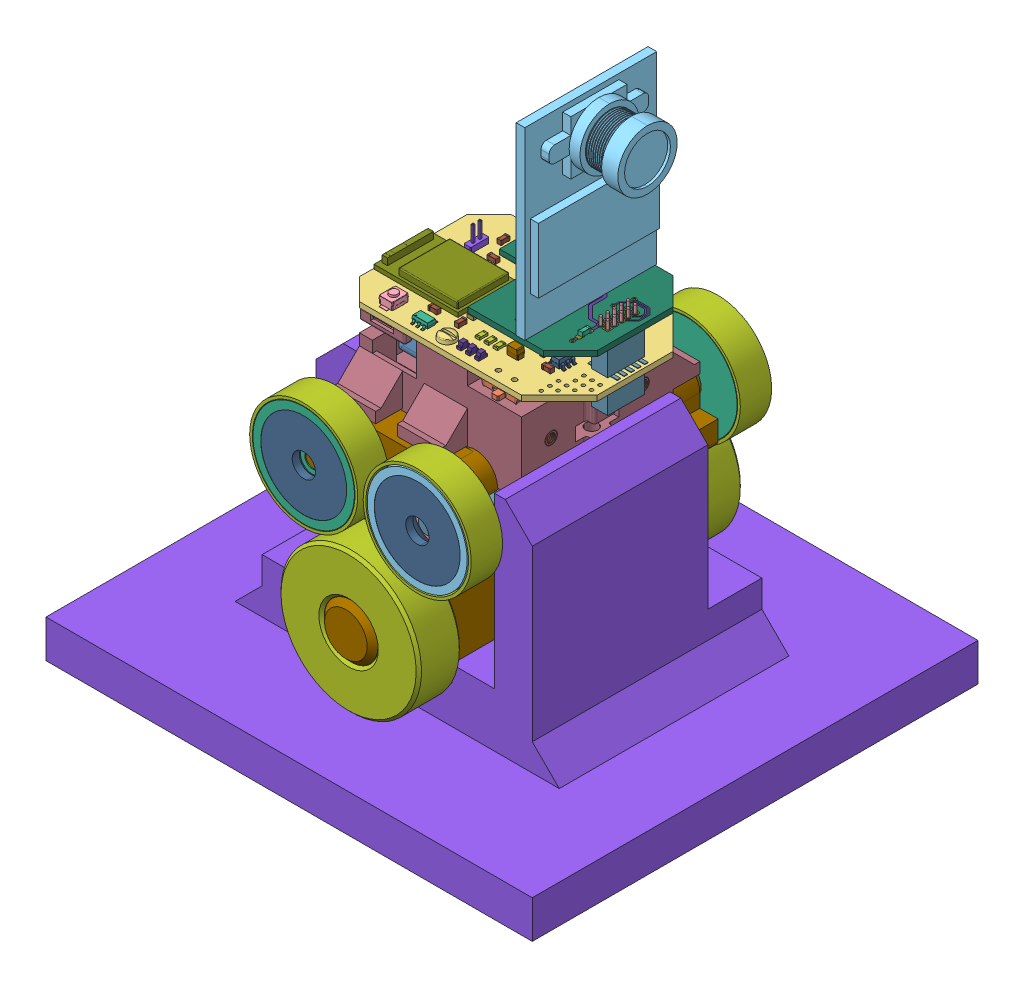
SolidWorks assembly life_time_test, configuration Default. Lengths in mm.
Overall size (90 100.86 82.5).
164 component instances, 45 part files, 11 mates.
Components (placement in the parent):
- AstroAnt_small_magnet-1: AstroAnt_small_magnet [Default] at (33.8115 12.6549 0.8712) size (45.75 69.7 55.6)
  - LiPo_360mAh-1: LiPo_360mAh [Default] at (6.8166 4.9998 44.2756) size (25 7 18)
  - 92120A150_Brass Heat-Set Inserts for Plastic-1: 92120A150_Brass Heat-Set Inserts for Plastic [92120A150] at (19.9543 12.4998 45.7029) size (2.56 3.33 2.56)
  - 92120A150_Brass Heat-Set Inserts for Plastic-2: 92120A150_Brass Heat-Set Inserts for Plastic [92120A150] at (4.9543 12.4998 33.9529) size (2.56 3.33 2.56)
  - 92120A150_Brass Heat-Set Inserts for Plastic-3: 92120A150_Brass Heat-Set Inserts for Plastic [92120A150] at (4.9543 12.4998 57.4529) size (2.56 3.33 2.56)
  - 91460A005_METRIC CHEESE HEAD SLOTTED MACHINE SCREW-8: 91460A005_METRIC CHEESE HEAD SLOTTED MACHINE SCREW [91460A005] at (4.9543 14.9998 57.4529) x (1 0 0) z (0 1 0) size (3 3 7.1)
  - 91460A005_METRIC CHEESE HEAD SLOTTED MACHINE SCREW-9: 91460A005_METRIC CHEESE HEAD SLOTTED MACHINE SCREW [91460A005] at (4.9543 14.9998 33.9529) x (1 0 0) z (0 1 0) size (3 3 7.1)
  - 91460A005_METRIC CHEESE HEAD SLOTTED MACHINE SCREW-10: 91460A005_METRIC CHEESE HEAD SLOTTED MACHINE SCREW [91460A005] at (19.9543 14.9998 45.7029) x (1 0 0) z (0 1 0) size (3 3 7.1)
  - 92120A150_Brass Heat-Set Inserts for Plastic-4: 92120A150_Brass Heat-Set Inserts for Plastic [92120A150] at (4.9543 -0.6002 57.4529) x (-0.616962 0 -0.786993) z (0.786993 0 -0.616962) size (2.56 3.33 2.56)
  - 92120A150_Brass Heat-Set Inserts for Plastic-5: 92120A150_Brass Heat-Set Inserts for Plastic [92120A150] at (4.9543 -0.6002 33.9529) x (-0.616962 0 -0.786993) z (0.786993 0 -0.616962) size (2.56 3.33 2.56)
  - mainboard_v1.step-1: mainboard_v1.step [Default] at (-103.0457 13.9998 235.7029) x (0 0 -1) z (0 1 0) size (29.41 41 10.8)
    - B3U-1000P.step-1: B3U-1000P.step [Default] at (178.95 -97.38 1.05) x (1 0 0) z (0 -1 0) size (4 1.75 2.5)
      - COMPOUND.step-1: COMPOUND.step [Default] at origin size (4 1.75 2.5)
    - 20021321-00014C1LF.step-1: 20021321-00014C1LF.step [Default] at (190 -115.5 1.05) size (9.35 5.45 4.85)
      - COMPOUND-0.step-1: COMPOUND-0.step [Default] at origin size (9.35 5.45 4.85)
    - MP6513GJ-Z.step-1: MP6513GJ-Z.step [Default] at (201.21 -120 1.05) x (-1 0 0) z (0 0 1) size (2.8 2.9 1)
      - COMPOUND-1.step-1: COMPOUND-1.step [Default] at origin size (2.8 2.9 1)
    - MP6513GJ-Z.step-2: MP6513GJ-Z.step [Default] at (178.51 -103.46 1.05) size (2.8 2.9 1)
      - COMPOUND-1.step-1: COMPOUND-1.step [Default] at origin size (2.8 2.9 1)
    - R_0603_1608Metric.step-1: R_0603_1608Metric.step [Default] at (195.55 -104.38 -0.05) x (1 0 0) z (0 0 -1) size (1.6 0.8 0.45)
      - SOLID.step-1: SOLID.step [Default] at origin size (1.6 0.8 0.45)
    - R_0603_1608Metric.step-2: R_0603_1608Metric.step [Default] at (192.6 -99.86 -0.05) x (0 1 0) z (0 0 -1) size (1.6 0.8 0.45)
      - SOLID.step-1: SOLID.step [Default] at origin size (1.6 0.8 0.45)
    - PinHeader_2x01_P1.27mm_Vertical.step-1: PinHeader_2x01_P1.27mm_Vertical.step [Default] at (194.96 -96.07 1.05) size (3.4 1.27 6.3)
      - SOLID-2.step-1: SOLID-2.step [Default] at origin size (3.4 1.27 6.3)
    - TAJP106K010RNJ.step-1: TAJP106K010RNJ.step [Default] at (196.22 -98.14 -0.05) x (-1 0 0) z (0 0 -1) size (2.05 1.4 1.7)
      - COMPOUND-3.step-1: COMPOUND-3.step [Default] at origin size (2.05 1.4 1.7)
    - TAJP106K010RNJ.step-2: TAJP106K010RNJ.step [Default] at (181.68 -117.23 1.05) x (0 1 0) z (0 0 1) size (2.05 1.4 1.7)
      - COMPOUND-3.step-1: COMPOUND-3.step [Default] at origin size (2.05 1.4 1.7)
    - SOT-23-5.step-1: SOT-23-5.step [Default] at (195.38 -122.78 1.05) x (0 1 0) z (0 0 1) size (2.8 2.9 1.55)
      - SOLID-4.step-1: SOLID-4.step [Default] at origin size (2.8 2.9 1.55)
    - C_0603_1608Metric.step-1: C_0603_1608Metric.step [Default] at (192.91 -122.55 1.05) x (0 -1 0) z (0 0 1) size (1.6 0.8 0.8)
      - SOLID-5.step-1: SOLID-5.step [Default] at origin size (1.6 0.8 0.8)
    - C_0603_1608Metric.step-2: C_0603_1608Metric.step [Default] at (193.57 -119.76 1.05) size (1.6 0.8 0.8)
      - SOLID-5.step-1: SOLID-5.step [Default] at origin size (1.6 0.8 0.8)
    - ECS-.327-12.5-12-TR.step-1: ECS-.327-12.5-12-TR.step [Default] at (184.31 -107.18 1.05) size (2 1.2 0.7)
      - COMPOUND-6.step-1: COMPOUND-6.step [Default] at origin size (2 1.2 0.7)
    - C_0603_1608Metric.step-3: C_0603_1608Metric.step [Default] at (197.67 -113.69 1.05) size (1.6 0.8 0.8)
      - SOLID-5.step-1: SOLID-5.step [Default] at origin size (1.6 0.8 0.8)
    - C_0603_1608Metric.step-4: C_0603_1608Metric.step [Default] at (197.64 -107.18 1.05) size (1.6 0.8 0.8)
      - SOLID-5.step-1: SOLID-5.step [Default] at origin size (1.6 0.8 0.8)
    - C_0603_1608Metric.step-5: C_0603_1608Metric.step [Default] at (190.96 -108.09 1.05) x (0 1 0) z (0 0 1) size (1.6 0.8 0.8)
      - SOLID-5.step-1: SOLID-5.step [Default] at origin size (1.6 0.8 0.8)
    - 1734592-6.step-1: 1734592-6.step [Default] at (203.79 -118 -1.05) x (0 -1 0) z (1 0 0) size (8.43 2.05 5.11)
      - SOLID-7.step-1: SOLID-7.step [Default] at origin size (8.43 2.05 5.11)
    - 1734592-6.step-2: 1734592-6.step [Default] at (176.19 -98 -1.05) x (0 1 0) z (-1 0 0) size (8.43 2.05 5.11)
      - SOLID-7.step-1: SOLID-7.step [Default] at origin size (8.43 2.05 5.11)
    - 20021321-00010C4LF.step-1: 20021321-00010C4LF.step [Default] at (190 -127.85 -0.05) x (1 0 0) z (0 0 -1) size (6.81 5.45 4.85)
      - COMPOUND-8.step-1: COMPOUND-8.step [Default] at origin size (6.81 5.45 4.85)
    - 20021321-00010C4LF.step-2: 20021321-00010C4LF.step [Default] at (190 -127.85 1.05) size (6.81 5.45 4.85)
      - COMPOUND-8.step-1: COMPOUND-8.step [Default] at origin size (6.81 5.45 4.85)
    - C_0603_1608Metric.step-6: C_0603_1608Metric.step [Default] at (181.31 -102.6 1.05) x (0 -1 0) z (0 0 1) size (1.6 0.8 0.8)
      - SOLID-5.step-1: SOLID-5.step [Default] at origin size (1.6 0.8 0.8)
    - C_0603_1608Metric.step-7: C_0603_1608Metric.step [Default] at (198.25 -119.14 1.05) x (0 -1 0) z (0 0 1) size (1.6 0.8 0.8)
      - SOLID-5.step-1: SOLID-5.step [Default] at origin size (1.6 0.8 0.8)
    - MPU6050.step-1: MPU6050.step [Default] at (198.43 -101.5 1.05) x (0 1 0) z (1 0 0) size (4 0.95 4)
      - COMPOUND-9.step-1: COMPOUND-9.step [Default] at origin size (4 0.95 4)
    - C_0603_1608Metric.step-8: C_0603_1608Metric.step [Default] at (194.9 -99.89 1.05) x (0 -1 0) z (0 0 1) size (1.6 0.8 0.8)
      - SOLID-5.step-1: SOLID-5.step [Default] at origin size (1.6 0.8 0.8)
    - C_0603_1608Metric.step-9: C_0603_1608Metric.step [Default] at (201.98 -100.38 1.05) x (0 -1 0) z (0 0 1) size (1.6 0.8 0.8)
      - SOLID-5.step-1: SOLID-5.step [Default] at origin size (1.6 0.8 0.8)
    - C_0603_1608Metric.step-10: C_0603_1608Metric.step [Default] at (201.98 -103.78 1.05) x (0 1 0) z (0 0 1) size (1.6 0.8 0.8)
      - SOLID-5.step-1: SOLID-5.step [Default] at origin size (1.6 0.8 0.8)
    - C_0603_1608Metric.step-11: C_0603_1608Metric.step [Default] at (198.81 -97.82 1.05) size (1.6 0.8 0.8)
      - SOLID-5.step-1: SOLID-5.step [Default] at origin size (1.6 0.8 0.8)
    - SOT-23-5.step-2: SOT-23-5.step [Default] at (184.86 -122.77 1.05) x (0 1 0) z (0 0 1) size (2.8 2.9 1.55)
      - SOLID-4.step-1: SOLID-4.step [Default] at origin size (2.8 2.9 1.55)
    - SOT-23-5.step-3: SOT-23-5.step [Default] at (197.58 -110.46 1.05) x (0 1 0) z (0 0 1) size (2.8 2.9 1.55)
      - SOLID-4.step-1: SOLID-4.step [Default] at origin size (2.8 2.9 1.55)
    - MDBT50Q-1MV2.step-1: MDBT50Q-1MV2.step [Default] at (187.3136 -98.605 1.0754) x (-1 0 0) z (0 1 0) size (10.5 2.06 15.5)
      - SOLID-10.step-1: SOLID-10.step [Default] at origin size (10.5 2.06 15.5)
    - C_0603_1608Metric.step-12: C_0603_1608Metric.step [Default] at (189.44 -108.09 1.05) x (0 1 0) z (0 0 1) size (1.6 0.8 0.8)
      - SOLID-5.step-1: SOLID-5.step [Default] at origin size (1.6 0.8 0.8)
    - C_0603_1608Metric.step-13: C_0603_1608Metric.step [Default] at (181.57 -107.18 1.05) x (-1 0 0) z (0 0 1) size (1.6 0.8 0.8)
      - SOLID-5.step-1: SOLID-5.step [Default] at origin size (1.6 0.8 0.8)
    - C_0603_1608Metric.step-14: C_0603_1608Metric.step [Default] at (186.97 -107.18 1.05) size (1.6 0.8 0.8)
      - SOLID-5.step-1: SOLID-5.step [Default] at origin size (1.6 0.8 0.8)
    - C_0603_1608Metric.step-15: C_0603_1608Metric.step [Default] at (184.77 -119.75 1.05) x (-1 0 0) z (0 0 1) size (1.6 0.8 0.8)
      - SOLID-5.step-1: SOLID-5.step [Default] at origin size (1.6 0.8 0.8)
    - C_0603_1608Metric.step-16: C_0603_1608Metric.step [Default] at (182.37 -122.54 1.05) x (0 -1 0) z (0 0 1) size (1.6 0.8 0.8)
      - SOLID-5.step-1: SOLID-5.step [Default] at origin size (1.6 0.8 0.8)
    - LED_0603_1608Metric.step-1: LED_0603_1608Metric.step [Default] at (178.19 -111.01 1.05) size (1.6 0.8 1.1)
      - SOLID-11.step-1: SOLID-11.step [Default] at origin size (1.6 0.8 1.1)
    - LED_0603_1608Metric.step-2: LED_0603_1608Metric.step [Default] at (178.19 -112.66 1.05) size (1.6 0.8 1.1)
      - SOLID-11.step-1: SOLID-11.step [Default] at origin size (1.6 0.8 1.1)
    - LED_0603_1608Metric.step-3: LED_0603_1608Metric.step [Default] at (178.19 -114.31 1.05) size (1.6 0.8 1.1)
      - SOLID-11.step-1: SOLID-11.step [Default] at origin size (1.6 0.8 1.1)
    - LED_0603_1608Metric.step-4: LED_0603_1608Metric.step [Default] at (202.34 -112.21 1.05) x (0 1 0) z (0 0 1) size (1.6 0.8 1.1)
      - SOLID-11.step-1: SOLID-11.step [Default] at origin size (1.6 0.8 1.1)
    - 473460001.step-1: 473460001.step [Default] at (201.68 -99.72 -1.25) x (0 -1 0) z (1 0 0) size (7.98 2.94 5.43)
      - COMPOUND-12.step-1: COMPOUND-12.step [Default] at origin size (7.98 2.94 5.43)
    - L_0603_1608Metric.step-1: L_0603_1608Metric.step [Default] at (192.48 -108.09 1.05) x (0 1 0) z (0 0 1) size (1.6 0.8 0.8)
      - SOLID-13.step-1: SOLID-13.step [Default] at origin size (1.6 0.8 0.8)
    - R_0603_1608Metric.step-3: R_0603_1608Metric.step [Default] at (185.18 -111.31 1.05) x (-1 0 0) z (0 0 1) size (1.6 0.8 0.45)
      - SOLID.step-1: SOLID.step [Default] at origin size (1.6 0.8 0.45)
    - R_0603_1608Metric.step-4: R_0603_1608Metric.step [Default] at (185.18 -109.77 1.05) size (1.6 0.8 0.45)
      - SOLID.step-1: SOLID.step [Default] at origin size (1.6 0.8 0.45)
    - R_0603_1608Metric.step-5: R_0603_1608Metric.step [Default] at (181.62 -111.01 1.05) size (1.6 0.8 0.45)
      - SOLID.step-1: SOLID.step [Default] at origin size (1.6 0.8 0.45)
    - R_0603_1608Metric.step-6: R_0603_1608Metric.step [Default] at (181.62 -112.66 1.05) size (1.6 0.8 0.45)
      - SOLID.step-1: SOLID.step [Default] at origin size (1.6 0.8 0.45)
    - R_0603_1608Metric.step-7: R_0603_1608Metric.step [Default] at (181.62 -114.31 1.05) x (-1 0 0) z (0 0 1) size (1.6 0.8 0.45)
      - SOLID.step-1: SOLID.step [Default] at origin size (1.6 0.8 0.45)
    - R_0603_1608Metric.step-8: R_0603_1608Metric.step [Default] at (194.84 -108.1 1.05) x (0 1 0) z (0 0 1) size (1.6 0.8 0.45)
      - SOLID.step-1: SOLID.step [Default] at origin size (1.6 0.8 0.45)
    - R_0603_1608Metric.step-9: R_0603_1608Metric.step [Default] at (200.69 -112.2325 1.05) x (0 1 0) z (0 0 1) size (1.6 0.8 0.45)
      - SOLID.step-1: SOLID.step [Default] at origin size (1.6 0.8 0.45)
    - R_0603_1608Metric.step-10: R_0603_1608Metric.step [Default] at (196.22 -101.51 -0.05) x (-1 0 0) z (0 0 -1) size (1.6 0.8 0.45)
      - SOLID.step-1: SOLID.step [Default] at origin size (1.6 0.8 0.45)
    - R_0603_1608Metric.step-11: R_0603_1608Metric.step [Default] at (196.22 -99.9725 -0.05) x (-1 0 0) z (0 0 -1) size (1.6 0.8 0.45)
      - SOLID.step-1: SOLID.step [Default] at origin size (1.6 0.8 0.45)
    - SW_SPDT_PCM12.step-1: SW_SPDT_PCM12.step [Default] at (178.18 -119.37 -0.05) x (0 1 0) z (0 0 -1) size (7.7 5 2)
      - SOLID-14.step-1: SOLID-14.step [Default] at origin size (7.7 5 2)
    - COMPOUND-15.step-1: COMPOUND-15.step [Default] at origin size (28 41 1)
  - ball_bearing_5x11x4mm-1: ball_bearing_5x11x4mm [Default] at (-65.9801 -4.7758 21.2029) x (0.999925 -0.012245 0) z (0 0 1) size (8 8 2.5)
  - wheel_holder_non_motor-1: wheel_holder_non_motor [Default] at (-90.7699 -0.8362 17.9029) size (18.5 18.5 5.8)
  - wheel_holder_non_motor-2: wheel_holder_non_motor [Default] at (1.3792 -86.6559 73.5029) x (0.185441 0.982655 0) z (0 0 -1) size (18.5 18.5 5.8)
  - ball_bearing_5x11x4mm-2: ball_bearing_5x11x4mm [Default] at (-9.788 -57.5376 70.2029) x (0.373101 0.927791 0) z (0 0 -1) size (8 8 2.5)
  - wheel_motor-1: wheel_motor [Default] at (44.5289 -0.8963 17.9029) size (18.8 18.8 5.8)
  - wheel_motor-2: wheel_motor [Default] at (-4.9746 26.526 73.5029) x (-0.038296 0.999266 0) z (0 0 -1) size (18.8 18.8 5.8)
  - tire-1: tire [Default] at (58.6593 -4.042 17.9029) size (20 20 5.8)
  - tire-2: tire [Default] at (37.6493 -4.042 17.9029) size (20 20 5.8)
  - tire-3: tire [Default] at (58.6593 -4.042 67.7029) size (20 20 5.8)
  - tire-4: tire [Default] at (37.6493 -4.042 67.7029) size (20 20 5.8)
  - PA2-50_with_gearbox-3: PA2-50_with_gearbox [Default] at (45.51 -3.6027 60.1029) x (-1 0 0) z (0 0 1) size (30.92 12.52 38.5)
    - PA2-50-1: PA2-50 [Default] at (26.117 -19.7771 -19.1) x (0 0 1) z (0.954024 0.299729 0) size (29.1 8 8)
    - gearbox-1: gearbox [Default] at origin size (29.9 11.5 13.6)
  - PA2-50_with_gearbox-4: PA2-50_with_gearbox [Default] at (-35.6268 -3.6027 31.3029) x (1 0 0) z (0 0 -1) size (30.92 12.52 38.5)
    - PA2-50-1: PA2-50 [Default] at (26.117 -19.7771 -19.1) x (0 0 1) z (0.954024 0.299729 0) size (29.1 8 8)
    - gearbox-1: gearbox [Default] at origin size (29.9 11.5 13.6)
  - RA22CS-N-1: RA22CS-N [Default] at (15.4466 -2.6002 19.5154) x (1 0 0) z (0 -1 0) size (15.88 3.17 15.88)
  - RA22CS-N-2: RA22CS-N [Default] at (-5.5634 -2.6002 19.5154) x (1 0 0) z (0 -1 0) size (15.88 3.17 15.88)
  - RA22CS-N-3: RA22CS-N [Default] at (-5.5634 -2.6002 71.8904) x (-0.968047 -0.250767 0) z (0.250767 -0.968047 0) size (15.88 3.17 15.88)
  - RA22CS-N-4: RA22CS-N [Default] at (15.4466 -2.6002 71.8904) x (-0.968047 -0.250767 0) z (0.250767 -0.968047 0) size (15.88 3.17 15.88)
  - TPiS_1084-1: TPiS_1084 [Default] at (-17.7438 -7.4002 31.4743) size (9.3 10.3 10.11)
  - IR_TEMP_module-1: IR_TEMP_module [Default] at (15.0895 3.8498 50.7532) x (0 0 -1) z (0 1 0) size (10 20 1.85)
  - robobody-1: robobody [Default] at (-9.0457 6.9406 -0.9986) size (31.5 16.1 38)
  - 92120A150_Brass Heat-Set Inserts for Plastic-6: 92120A150_Brass Heat-Set Inserts for Plastic [92120A150] at (19.9543 -0.6002 45.7029) x (-0.616962 0 -0.786993) z (0.786993 0 -0.616962) size (2.56 3.33 2.56)
  - motor_holder_2-1: motor_holder_2 [Default] at (52.4112 -9.4002 -5.2676) size (31.5 8.8 52.2)
  - 92120A150_Brass Heat-Set Inserts for Plastic-7: 92120A150_Brass Heat-Set Inserts for Plastic [92120A150] at (19.4543 5.3998 54.2029) x (0 1 0) z (0 0 1) size (2.56 3.33 2.56)
  - 92120A150_Brass Heat-Set Inserts for Plastic-8: 92120A150_Brass Heat-Set Inserts for Plastic [92120A150] at (19.4543 5.3998 37.2029) x (0 1 0) z (0 0 1) size (2.56 3.33 2.56)
  - Camera1-Camera.step-1: Camera1-Camera.step [Default] at (-70.9957 22.1998 197.7029) x (0 0 -1) z (0 1 0) size (24.4 21.18 39.4)
    - Board_Geoms_150e.step-1: Board_Geoms_150e.step [Default] at origin size (24 19 1.05)
      - Pcb_150e.step-1: Pcb_150e.step [Default] at origin size (24 19 1)
      - topPads_150e.step-1: topPads_150e.step [Default] at (0 0 0.02) size (19.49 14.67 0.01)
      - topTracks_150e.step-1: topTracks_150e.step [Default] at (0 0 0.01) size (12.72 10.5 0.01)
      - botPads_150e.step-1: botPads_150e.step [Default] at (0 0 -1.02) size (19.49 14.67 0.01)
      - botTracks_150e.step-1: botTracks_150e.step [Default] at (0 0 -1.01) size (18.04 10.2 0.01)
      - botZones_150e.step-1: botZones_150e.step [Default] at (0 0 -1.01) size (23.45 18.45 0.01)
    - Step_Models_150e.step-1: Step_Models_150e.step [Default] at origin size (24.4 19.37 39.4)
      - Top_150e.step-1: Top_150e.step [Default] at origin size (24.4 19.37 39.4)
        - J2_ASSEMBLY_61432F3D.step-1: J2_ASSEMBLY_61432F3D.step [Default] at (149.47 -82.87 -1) x (1 0 0) z (0 0 -1) size (6.35 3.4 6.9)
          - Body.step-1: Body.step [Default] at origin size (6.35 3.4 1.3)
          - LeadsArray.step-1: LeadsArray.step [Default] at origin size (5.58 1.77 6.9)
        - J2_ASSEMBLY_61432F3D.step-2: J2_ASSEMBLY_61432F3D.step [Default] at (149.46 -95.165 -1) x (1 0 0) z (0 0 -1) size (6.35 3.4 6.9)
          - Body.step-1: Body.step [Default] at origin size (6.35 3.4 1.3)
          - LeadsArray.step-1: LeadsArray.step [Default] at origin size (5.58 1.77 6.9)
        - U1_Arducam_OV2640_61432450.step-1: U1_Arducam_OV2640_61432450.step [Default] at (150.125 -88.26 0) x (-1 0 0) z (0 0 1) size (24.4 13.6 34.1)
        - C1_C_0603_1608Metric_61432400.step-1: C1_C_0603_1608Metric_61432400.step [Default] at (146.47 -95.15 0) x (-1 0 0) z (0 0 1) size (1.6 0.8 0.8)
- 26_10_8_bearing-1: 26_10_8_bearing [Default] at (38.7531 -10.4061 16.5741) size (26 26 8)
- 26_10_8_bearing-2: 26_10_8_bearing [Default] at (38.7531 -10.4061 68.5741) size (26 26 8)
- base_2-1: base_2 [Default] at (13.7531 1.3417 -0.5) size (90 48.34 82.5)
- base_1-4: base_1 [Default] at (28.7531 -0.7761 -1.5923) size (20 15 30)
- base_1-5: base_1 [Default] at (48.7531 -0.7761 94.7404) x (-1 0 0) z (0 0 -1) size (20 15 30)
Mates (geometry in assembly coordinates):
- Coincident1: coincident aligned: plane of AstroAnt_small_magnet-1/wheel_holder_non_motor-1 through (28.2481 10.0547 24.5741) normal (0 0 1); plane of 26_10_8_bearing-1 through (38.7531 -10.4061 24.5741) normal (0 0 1)
- Tangent3: tangent anti-aligned: cylinder of AstroAnt_small_magnet-1/tire-1 through (49.2581 10.0547 24.5741) axis (0 0 -1) radius 10; cylinder of 26_10_8_bearing-1 through (38.7531 -10.4061 24.5741) axis (0 0 -1) radius 13
- Tangent4: tangent anti-aligned: cylinder of AstroAnt_small_magnet-1/tire-2 through (28.2481 10.0547 24.5741) axis (0 0 -1) radius 10; cylinder of 26_10_8_bearing-1 through (38.7531 -10.4061 24.5741) axis (0 0 -1) radius 13
- Coincident2: coincident aligned: plane of AstroAnt_small_magnet-1/wheel_motor-2 through (28.2481 10.0547 68.5741) normal (0 0 -1); plane of 26_10_8_bearing-2 through (38.7531 -10.4061 68.5741) normal (0 0 -1)
- Tangent5: tangent anti-aligned: cylinder of AstroAnt_small_magnet-1/tire-4 through (28.2481 10.0547 74.3741) axis (0 0 -1) radius 10; cylinder of 26_10_8_bearing-2 through (38.7531 -10.4061 76.5741) axis (0 0 -1) radius 13
- Tangent6: tangent anti-aligned: cylinder of AstroAnt_small_magnet-1/tire-3 through (49.2581 10.0547 74.3741) axis (0 0 -1) radius 10; cylinder of 26_10_8_bearing-2 through (38.7531 -10.4061 76.5741) axis (0 0 -1) radius 13
- Concentric12: concentric aligned: cylinder of base_2-1 through (38.7531 -31.9061 35.5741) axis (0 1 0) radius 2.75; cylinder of base_1-4 through (38.7531 -17.9061 35.5741) axis (0 1 0) radius 2.2
- Concentric13: concentric aligned: cylinder of base_2-1 through (38.7531 -31.9061 57.5741) axis (0 1 0) radius 2.75; cylinder of base_1-5 through (38.7531 -7.9061 57.5741) axis (0 1 0) radius 4.25
- Coincident14: coincident anti-aligned: plane of base_2-1 through (63.7531 -17.9061 25.0741) normal (0 1 0); plane of base_1-4 through (48.7531 -17.9061 25.0741) normal (0 -1 0)
- Coincident15: coincident anti-aligned: plane of base_2-1 through (63.7531 -17.9061 25.0741) normal (0 1 0); plane of base_1-5 through (28.7531 -17.9061 68.0741) normal (0 -1 0)
- Parallel9: parallel anti-aligned: plane of base_2-1 through (48.8531 -14.9061 67.5741) normal (-1 0 0); plane of base_1-5 through (48.7531 -0.7761 94.7404) normal (1 0 0)
